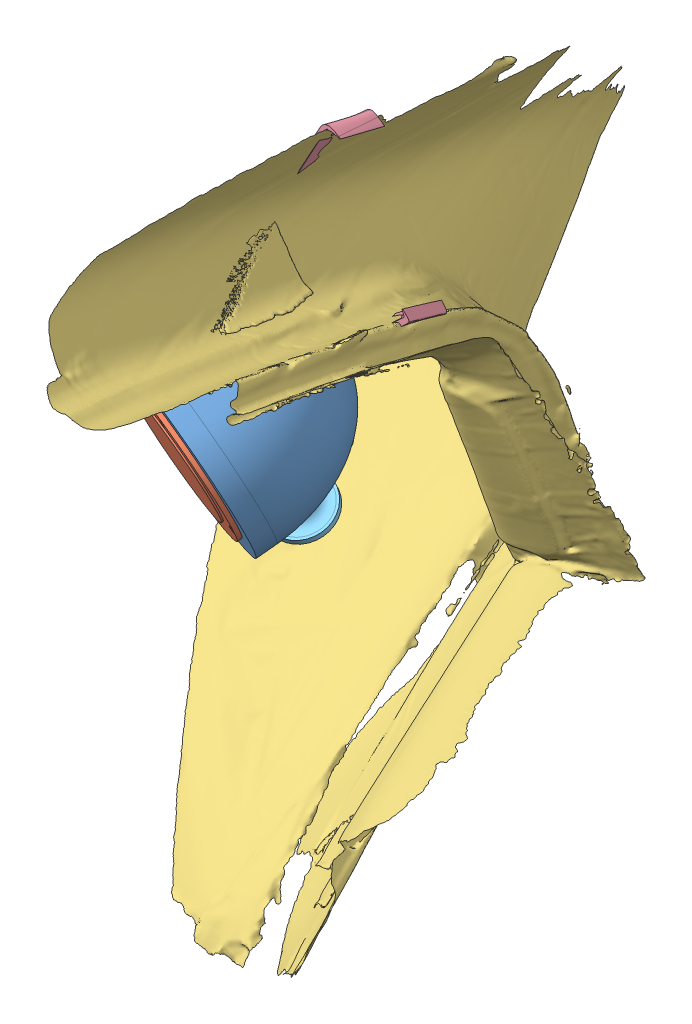
SolidWorks assembly 汽车音箱组装, configuration Default. Lengths in mm.
Overall size (276.78 374.21 467.74).
5 component instances, 5 part files, 3 mates.
Components (placement in the parent):
- 汽车音箱-1: 汽车音箱 [Default] at (-113.354 114.134 147.2243) x (-0.153505 -0.858689 -0.488968) z (0.937484 -0.282967 0.202617) size (112.81 81.35 112.81)
- 莞音3寸圆-1: 莞音3寸圆 [Default] at (-114.1349 113.0658 149.3454) x (0.904567 -0.406586 0.128241) z (0.290169 0.80753 0.513514) size (89 52 89)
- focus_a-1: focus_a [Default] at (-114.0656 67.5174 400.1558) size (276.78 370.21 467.74)
- focus_a_a_clear-1: focus_a_a_clear [默认] at (-120.6332 55.148 366.9388) size (84.04 114.17 30.22)
- 音箱支架-1: 音箱支架 [默认] at (-111.3135 116.9255 141.6816) x (-0.189681 -0.847091 -0.496445) z (0.930839 -0.315997 0.183536) size (88.69 66.4 89.69)
Mates (geometry in assembly coordinates):
- Concentric1: concentric anti-aligned: cylinder of 汽车音箱-1 through (-112.417 115.4159 144.6789) axis (-0.312347 -0.427297 0.848444) radius 36.5; cone of 莞音3寸圆-1 through (-113.354 114.134 147.2243) axis (0.312347 0.427297 -0.848444)
- Coincident1: coincident anti-aligned: plane of 汽车音箱-1 through (-113.354 114.134 147.2243) normal (-0.312347 -0.427297 0.848444); plane of 莞音3寸圆-1 through (-113.354 114.134 147.2243) normal (0.312347 0.427297 -0.848444)
- 锁定1: lock: unknown of 汽车音箱-1; unknown of 音箱支架-1
